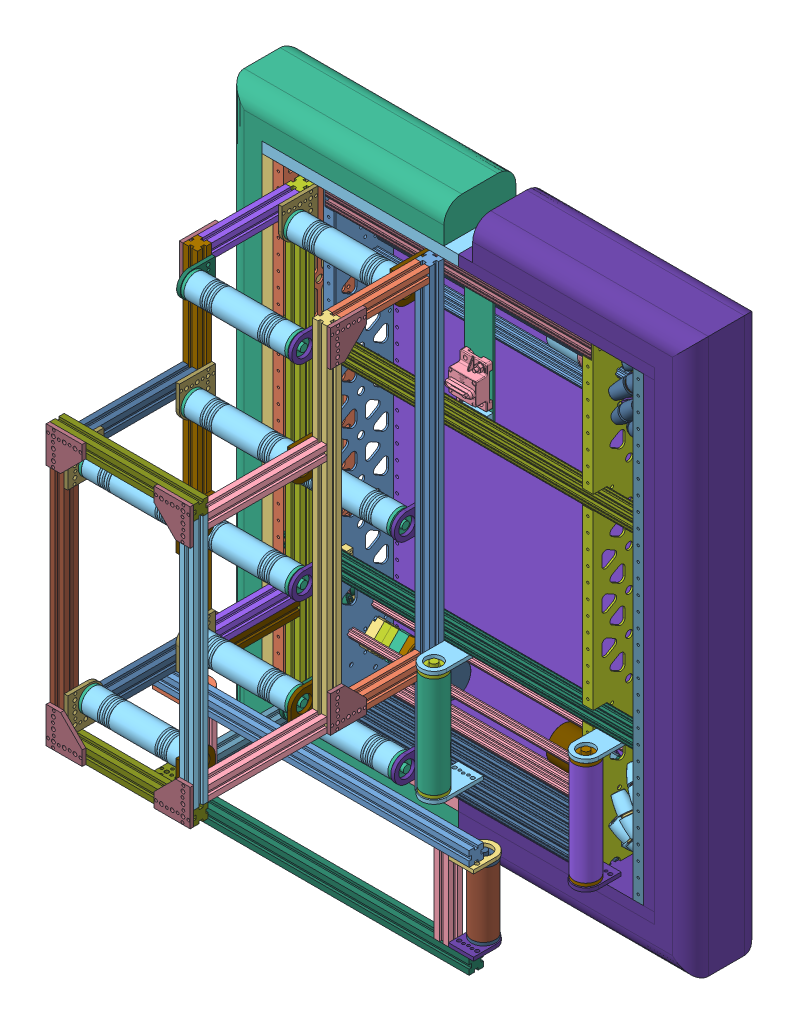
SolidWorks assembly Robot 2020, configuration Default. Lengths in mm. (continued)
Components (placement in the parent): (continued)
- Copy of Fame 2020-1: Copy of Fame 2020 [Default] at origin size (819.15 977.9 171.99) (continued)
  - NEO Gearbox 2-stage Custom v5(Mirror)^Copy of Fame 2020-1: NEO Gearbox 2-stage Custom v5(Mirror)^Copy of Fame 2020 [Default] at (0 0 425) x (-1 0 0) z (0 0 -1) size (164.9 90.53 90.53) (virtual) (continued)
    - VersaPlanetary_4_1_Gear_Kit_217-2818 v1(Mirror)^NEO Gearbox 2-stage Custom v5(Mirror)_Copy of Fame 2020-1: VersaPlanetary_4_1_Gear_Kit_217-2818 v1(Mirror)^NEO Gearbox 2-stage Custom v5(Mirror)_Copy of Fame 2020 [Default] at (-15.25 22.225 0) x (0 -0.707107 -0.707107) z (1 0 0) size (35.49 35.49 17.4) (virtual) (continued)
      - 217-2725-002 Rev1_24t Planet(Mirror)^VersaPlanetary_4_1_Gear_Kit_217-2818 v1(Mirror)_NEO Gearbox 2-stage Custom v5(Mirror)_Copy of Fame 2020-1: 217-2725-002 Rev1_24t Planet(Mirror)^VersaPlanetary_4_1_Gear_Kit_217-2818 v1(Mirror)_NEO Gearbox 2-stage Custom v5(Mirror)_Copy of Fame 2020 [Default] at (-45.2382 -525.6819 212.025) x (-0.793353 0.608761 0) z (0 0 -1) size (13.12 13.1 8) (virtual)
      - 217-2725-002 Rev1_24t Planet(Mirror)^VersaPlanetary_4_1_Gear_Kit_217-2818 v1(Mirror)_NEO Gearbox 2-stage Custom v5(Mirror)_Copy of Fame 2020-2: 217-2725-002 Rev1_24t Planet(Mirror)^VersaPlanetary_4_1_Gear_Kit_217-2818 v1(Mirror)_NEO Gearbox 2-stage Custom v5(Mirror)_Copy of Fame 2020 [Default] at (-28.1418 -525.6819 212.025) x (-0.608761 -0.793353 0) z (0 0 -1) size (13.12 13.1 8) (virtual)
      - 217-2725-002 Rev1_24t Planet(Mirror)^VersaPlanetary_4_1_Gear_Kit_217-2818 v1(Mirror)_NEO Gearbox 2-stage Custom v5(Mirror)_Copy of Fame 2020-3: 217-2725-002 Rev1_24t Planet(Mirror)^VersaPlanetary_4_1_Gear_Kit_217-2818 v1(Mirror)_NEO Gearbox 2-stage Custom v5(Mirror)_Copy of Fame 2020 [Default] at (-28.1418 -508.5855 212.025) x (0.793353 -0.608761 0) z (0 0 -1) size (13.12 13.1 8) (virtual)
      - 217-2725-002 Rev1_24t Planet(Mirror)^VersaPlanetary_4_1_Gear_Kit_217-2818 v1(Mirror)_NEO Gearbox 2-stage Custom v5(Mirror)_Copy of Fame 2020-4: 217-2725-002 Rev1_24t Planet(Mirror)^VersaPlanetary_4_1_Gear_Kit_217-2818 v1(Mirror)_NEO Gearbox 2-stage Custom v5(Mirror)_Copy of Fame 2020 [Default] at (-45.2382 -508.5855 212.025) x (0.608761 0.793353 0) z (0 0 -1) size (13.12 13.1 8) (virtual)
      - 217-2724-002 Rev1(Mirror)^VersaPlanetary_4_1_Gear_Kit_217-2818 v1(Mirror)_NEO Gearbox 2-stage Custom v5(Mirror)_Copy of Fame 2020-1: 217-2724-002 Rev1(Mirror)^VersaPlanetary_4_1_Gear_Kit_217-2818 v1(Mirror)_NEO Gearbox 2-stage Custom v5(Mirror)_Copy of Fame 2020 [Default] at (-36.69 -517.1337 218.375) x (1 0 0) z (0 0 -1) size (34.7 34.7 4.7) (virtual)
      - 217-2625-010 Rev1(Mirror)^VersaPlanetary_4_1_Gear_Kit_217-2818 v1(Mirror)_NEO Gearbox 2-stage Custom v5(Mirror)_Copy of Fame 2020-1: 217-2625-010 Rev1(Mirror)^VersaPlanetary_4_1_Gear_Kit_217-2818 v1(Mirror)_NEO Gearbox 2-stage Custom v5(Mirror)_Copy of Fame 2020 [Default] at (-45.2382 -525.6819 214.725) x (0.854322 0.519745 0) z (0 0 1) size (4 4 12) (virtual)
      - 217-2625-010 Rev1(Mirror)^VersaPlanetary_4_1_Gear_Kit_217-2818 v1(Mirror)_NEO Gearbox 2-stage Custom v5(Mirror)_Copy of Fame 2020-2: 217-2625-010 Rev1(Mirror)^VersaPlanetary_4_1_Gear_Kit_217-2818 v1(Mirror)_NEO Gearbox 2-stage Custom v5(Mirror)_Copy of Fame 2020 [Default] at (-28.1418 -525.6819 214.725) x (-0.519745 0.854322 0) z (0 0 1) size (4 4 12) (virtual)
      - 217-2625-010 Rev1(Mirror)^VersaPlanetary_4_1_Gear_Kit_217-2818 v1(Mirror)_NEO Gearbox 2-stage Custom v5(Mirror)_Copy of Fame 2020-3: 217-2625-010 Rev1(Mirror)^VersaPlanetary_4_1_Gear_Kit_217-2818 v1(Mirror)_NEO Gearbox 2-stage Custom v5(Mirror)_Copy of Fame 2020 [Default] at (-28.1418 -508.5855 214.725) x (-0.854322 -0.519745 0) z (0 0 1) size (4 4 12) (virtual)
      - 217-2625-010 Rev1(Mirror)^VersaPlanetary_4_1_Gear_Kit_217-2818 v1(Mirror)_NEO Gearbox 2-stage Custom v5(Mirror)_Copy of Fame 2020-4: 217-2625-010 Rev1(Mirror)^VersaPlanetary_4_1_Gear_Kit_217-2818 v1(Mirror)_NEO Gearbox 2-stage Custom v5(Mirror)_Copy of Fame 2020 [Default] at (-45.2382 -508.5855 214.725) x (0.519745 -0.854322 0) z (0 0 1) size (4 4 12) (virtual)
    - 217-2625-026 Rev1(Mirror)^NEO Gearbox 2-stage Custom v5(Mirror)_Copy of Fame 2020-1: 217-2625-026 Rev1(Mirror)^NEO Gearbox 2-stage Custom v5(Mirror)_Copy of Fame 2020 [Default] at (211.875 -317.5 391.6125) x (0 -0.707107 -0.707107) z (1 0 0) size (44.45 42 18.12) (virtual)
    - 217-2742-001 Rev4(Mirror)^NEO Gearbox 2-stage Custom v5(Mirror)_Copy of Fame 2020-1: 217-2742-001 Rev4(Mirror)^NEO Gearbox 2-stage Custom v5(Mirror)_Copy of Fame 2020 [Default] at (218.5752 -317.5 391.6125) x (1 0 0) z (0 -0.63857 0.769564) size (7 28 28) (virtual)
    - 217-2742-001 Rev4(Mirror)^NEO Gearbox 2-stage Custom v5(Mirror)_Copy of Fame 2020-2: 217-2742-001 Rev4(Mirror)^NEO Gearbox 2-stage Custom v5(Mirror)_Copy of Fame 2020 [Default] at (226.5752 -317.5 391.6125) x (1 0 0) z (0 -0.707107 0.707107) size (7 28 28) (virtual)
    - 217-2625-017 Rev1_9714K61(Mirror)^NEO Gearbox 2-stage Custom v5(Mirror)_Copy of Fame 2020-1: 217-2625-017 Rev1_9714K61(Mirror)^NEO Gearbox 2-stage Custom v5(Mirror)_Copy of Fame 2020 [Default] at (225.795 -317.6887 391.9075) x (0 0.983393 -0.181491) z (0 0.181491 0.983393) size (28.51 4.98 27.43) (virtual)
    - 217-2625-025 Rev1(Mirror)^NEO Gearbox 2-stage Custom v5(Mirror)_Copy of Fame 2020-1: 217-2625-025 Rev1(Mirror)^NEO Gearbox 2-stage Custom v5(Mirror)_Copy of Fame 2020 [Default] at (182.475 -317.5 391.6125) x (0 -0.707107 -0.707107) z (1 0 0) size (44.45 42 18) (virtual)
    - 217-2816-001 Rev1(Mirror)^NEO Gearbox 2-stage Custom v5(Mirror)_Copy of Fame 2020-1: 217-2816-001 Rev1(Mirror)^NEO Gearbox 2-stage Custom v5(Mirror)_Copy of Fame 2020 [Default] at (212.025 -317.5 391.6125) x (0 -0.707107 -0.707107) z (-1 0 0) size (42 42 14.5) (virtual)
    - 217-2816-001 Rev1(Mirror)^NEO Gearbox 2-stage Custom v5(Mirror)_Copy of Fame 2020-2: 217-2816-001 Rev1(Mirror)^NEO Gearbox 2-stage Custom v5(Mirror)_Copy of Fame 2020 [Default] at (199.325 -317.5 391.6125) x (0 -0.707107 -0.707107) z (-1 0 0) size (42 42 14.5) (virtual)
    - 217-4649-001 Rev1(Mirror)^NEO Gearbox 2-stage Custom v5(Mirror)_Copy of Fame 2020-1: 217-4649-001 Rev1(Mirror)^NEO Gearbox 2-stage Custom v5(Mirror)_Copy of Fame 2020 [Default] at (185.629 -317.5 391.6125) x (0 -0.707107 -0.707107) z (-1 0 0) size (18 18 13) (virtual)
    - VersaPlanetary_CIM_Adapter_217-4018 v1(Mirror)^NEO Gearbox 2-stage Custom v5(Mirror)_Copy of Fame 2020-1: VersaPlanetary_CIM_Adapter_217-4018 v1(Mirror)^NEO Gearbox 2-stage Custom v5(Mirror)_Copy of Fame 2020 [Default] at (165.15 -317.5 391.6125) x (0 -0.707107 -0.707107) z (0 -0.707107 0.707107) size (64.01 21.55 64.01) (virtual)
    - NEO Motor REV-21-1650 v2(Mirror)^NEO Gearbox 2-stage Custom v5(Mirror)_Copy of Fame 2020-1: NEO Motor REV-21-1650 v2(Mirror)^NEO Gearbox 2-stage Custom v5(Mirror)_Copy of Fame 2020 [Default] at (153.625 -317.5 391.6125) x (0 -0.707107 0.707107) z (-1 0 0) size (61.14 61.02 93.25) (virtual)
    - 3_1 Output Shaft Custom v6(Mirror)^NEO Gearbox 2-stage Custom v5(Mirror)_Copy of Fame 2020-1: 3_1 Output Shaft Custom v6(Mirror)^NEO Gearbox 2-stage Custom v5(Mirror)_Copy of Fame 2020 [Default] at (211.3752 -317.5 391.6125) x (1 0 0) z (0 -0.707107 0.707107) size (48.9 34.7 34.7) (virtual)
  - Left Wheel Assembly v4(Mirror)^Copy of Fame 2020-1: Left Wheel Assembly v4(Mirror)^Copy of Fame 2020 [Default] at (-500 0 0) x (-1 0 0) z (0 0 -1) size (65.82 166.11 165.01) (virtual)
    - 6_Mecanum_Wheel_Left_217-2799 v1(Mirror)^Left Wheel Assembly v4(Mirror)_Copy of Fame 2020-1: 6_Mecanum_Wheel_Left_217-2799 v1(Mirror)^Left Wheel Assembly v4(Mirror)_Copy of Fame 2020 [Default] x (0 0 -1) z (1 0 0) size (165.01 166.11 65.82) (virtual)
      - 217-2799-001 Rev1(Mirror)^6_Mecanum_Wheel_Left_217-2799 v1(Mirror)_Left Wheel Assembly v4(Mirror)_Copy of Fame 2020-1: 217-2799-001 Rev1(Mirror)^6_Mecanum_Wheel_Left_217-2799 v1(Mirror)_Left Wheel Assembly v4(Mirror)_Copy of Fame 2020 [Default] at (33.3875 -317.5 -234.0098) x (0.707107 0.707107 0) z (0 0 1) size (95.78 100.46 28.55) (virtual)
      - 217-2799-001 Rev1(Mirror)^6_Mecanum_Wheel_Left_217-2799 v1(Mirror)_Left Wheel Assembly v4(Mirror)_Copy of Fame 2020-2: 217-2799-001 Rev1(Mirror)^6_Mecanum_Wheel_Left_217-2799 v1(Mirror)_Left Wheel Assembly v4(Mirror)_Copy of Fame 2020 [Default] at (33.3875 -317.5 -221.3098) x (-0.987688 -0.156434 0) z (0 0 -1) size (95.78 100.46 28.55) (virtual)
      - 217-2799-002 Rev1(Mirror)^6_Mecanum_Wheel_Left_217-2799 v1(Mirror)_Left Wheel Assembly v4(Mirror)_Copy of Fame 2020-1: 217-2799-002 Rev1(Mirror)^6_Mecanum_Wheel_Left_217-2799 v1(Mirror)_Left Wheel Assembly v4(Mirror)_Copy of Fame 2020 [Default] at (4.057 -346.8305 -227.6598) x (-0.707107 0.707107 0) z (0.707107 0.707107 0) size (26.84 25.39 30.1) (virtual)
      - 217-2799-002 Rev1(Mirror)^6_Mecanum_Wheel_Left_217-2799 v1(Mirror)_Left Wheel Assembly v4(Mirror)_Copy of Fame 2020-2: 217-2799-002 Rev1(Mirror)^6_Mecanum_Wheel_Left_217-2799 v1(Mirror)_Left Wheel Assembly v4(Mirror)_Copy of Fame 2020 [Default] at (-7.5815 -323.9888 -227.6598) x (-0.156434 0.987688 0) z (0.987688 0.156434 0) size (26.84 25.39 30.1) (virtual)
      - 217-2799-002 Rev1(Mirror)^6_Mecanum_Wheel_Left_217-2799 v1(Mirror)_Left Wheel Assembly v4(Mirror)_Copy of Fame 2020-3: 217-2799-002 Rev1(Mirror)^6_Mecanum_Wheel_Left_217-2799 v1(Mirror)_Left Wheel Assembly v4(Mirror)_Copy of Fame 2020 [Default] at (-3.5711 -298.6686 -227.6598) x (0.45399 0.891007 0) z (0.891007 -0.45399 0) size (26.84 25.39 30.1) (virtual)
      - 217-2799-002 Rev1(Mirror)^6_Mecanum_Wheel_Left_217-2799 v1(Mirror)_Left Wheel Assembly v4(Mirror)_Copy of Fame 2020-4: 217-2799-002 Rev1(Mirror)^6_Mecanum_Wheel_Left_217-2799 v1(Mirror)_Left Wheel Assembly v4(Mirror)_Copy of Fame 2020 [Default] at (14.5561 -280.5414 -227.6598) x (0.891007 0.45399 0) z (0.45399 -0.891007 0) size (26.84 25.39 30.1) (virtual)
      - 217-2799-002 Rev1(Mirror)^6_Mecanum_Wheel_Left_217-2799 v1(Mirror)_Left Wheel Assembly v4(Mirror)_Copy of Fame 2020-5: 217-2799-002 Rev1(Mirror)^6_Mecanum_Wheel_Left_217-2799 v1(Mirror)_Left Wheel Assembly v4(Mirror)_Copy of Fame 2020 [Default] at (39.8763 -276.531 -227.6598) x (0.987688 -0.156434 0) z (-0.156434 -0.987688 0) size (26.84 25.39 30.1) (virtual)
      - 217-2799-002 Rev1(Mirror)^6_Mecanum_Wheel_Left_217-2799 v1(Mirror)_Left Wheel Assembly v4(Mirror)_Copy of Fame 2020-6: 217-2799-002 Rev1(Mirror)^6_Mecanum_Wheel_Left_217-2799 v1(Mirror)_Left Wheel Assembly v4(Mirror)_Copy of Fame 2020 [Default] at (62.718 -288.1695 -227.6598) x (0.707107 -0.707107 0) z (-0.707107 -0.707107 0) size (26.84 25.39 30.1) (virtual)
      - 217-2799-002 Rev1(Mirror)^6_Mecanum_Wheel_Left_217-2799 v1(Mirror)_Left Wheel Assembly v4(Mirror)_Copy of Fame 2020-7: 217-2799-002 Rev1(Mirror)^6_Mecanum_Wheel_Left_217-2799 v1(Mirror)_Left Wheel Assembly v4(Mirror)_Copy of Fame 2020 [Default] at (74.3565 -311.0112 -227.6598) x (0.156434 -0.987688 0) z (-0.987688 -0.156434 0) size (26.84 25.39 30.1) (virtual)
      - 217-2799-002 Rev1(Mirror)^6_Mecanum_Wheel_Left_217-2799 v1(Mirror)_Left Wheel Assembly v4(Mirror)_Copy of Fame 2020-8: 217-2799-002 Rev1(Mirror)^6_Mecanum_Wheel_Left_217-2799 v1(Mirror)_Left Wheel Assembly v4(Mirror)_Copy of Fame 2020 [Default] at (70.3461 -336.3314 -227.6598) x (-0.45399 -0.891007 0) z (-0.891007 0.45399 0) size (26.84 25.39 30.1) (virtual)
      - 217-2799-002 Rev1(Mirror)^6_Mecanum_Wheel_Left_217-2799 v1(Mirror)_Left Wheel Assembly v4(Mirror)_Copy of Fame 2020-9: 217-2799-002 Rev1(Mirror)^6_Mecanum_Wheel_Left_217-2799 v1(Mirror)_Left Wheel Assembly v4(Mirror)_Copy of Fame 2020 [Default] at (52.2189 -354.4586 -227.6598) x (-0.891007 -0.45399 0) z (-0.45399 0.891007 0) size (26.84 25.39 30.1) (virtual)
      - 217-2799-002 Rev1(Mirror)^6_Mecanum_Wheel_Left_217-2799 v1(Mirror)_Left Wheel Assembly v4(Mirror)_Copy of Fame 2020-10: 217-2799-002 Rev1(Mirror)^6_Mecanum_Wheel_Left_217-2799 v1(Mirror)_Left Wheel Assembly v4(Mirror)_Copy of Fame 2020 [Default] at (26.8987 -358.469 -227.6598) x (-0.987688 0.156434 0) z (0.156434 0.987688 0) size (26.84 25.39 30.1) (virtual)
      - 217-2586-003 Rev2(Mirror)^6_Mecanum_Wheel_Left_217-2799 v1(Mirror)_Left Wheel Assembly v4(Mirror)_Copy of Fame 2020-1: 217-2586-003 Rev2(Mirror)^6_Mecanum_Wheel_Left_217-2799 v1(Mirror)_Left Wheel Assembly v4(Mirror)_Copy of Fame 2020 [Default] at (-13.4676 -358.6894 -223.6536) x (0.41944 0.854155 -0.30739) z (0.757674 -0.142894 0.636798) size (19.46 28.57 19.46) (virtual)
      - 217-2586-003 Rev2(Mirror)^6_Mecanum_Wheel_Left_217-2799 v1(Mirror)_Left Wheel Assembly v4(Mirror)_Copy of Fame 2020-2: 217-2586-003 Rev2(Mirror)^6_Mecanum_Wheel_Left_217-2799 v1(Mirror)_Left Wheel Assembly v4(Mirror)_Copy of Fame 2020 [Default] at (-7.8019 -364.3551 -231.666) x (0.847342 0.451134 0.280161) z (-0.17892 0.739241 -0.649238) size (19.46 28.57 19.46) (virtual)
      - 217-2586-003 Rev2(Mirror)^6_Mecanum_Wheel_Left_217-2799 v1(Mirror)_Left Wheel Assembly v4(Mirror)_Copy of Fame 2020-3: 217-2586-003 Rev2(Mirror)^6_Mecanum_Wheel_Left_217-2799 v1(Mirror)_Left Wheel Assembly v4(Mirror)_Copy of Fame 2020 [Default] at (-27.4761 -331.196 -231.666) x (0.950684 -0.13308 0.280161) z (0.289766 0.703225 -0.649238) size (19.46 28.57 19.46) (virtual)
      - 217-2586-003 Rev2(Mirror)^6_Mecanum_Wheel_Left_217-2799 v1(Mirror)_Left Wheel Assembly v4(Mirror)_Copy of Fame 2020-4: 217-2586-003 Rev2(Mirror)^6_Mecanum_Wheel_Left_217-2799 v1(Mirror)_Left Wheel Assembly v4(Mirror)_Copy of Fame 2020 [Default] at (-23.9025 -292.8056 -231.666) x (0.690897 -0.666462 0.280161) z (0.647771 0.398601 -0.649238) size (19.46 28.57 19.46) (virtual)
      - 217-2586-003 Rev2(Mirror)^6_Mecanum_Wheel_Left_217-2799 v1(Mirror)_Left Wheel Assembly v4(Mirror)_Copy of Fame 2020-5: 217-2586-003 Rev2(Mirror)^6_Mecanum_Wheel_Left_217-2799 v1(Mirror)_Left Wheel Assembly v4(Mirror)_Copy of Fame 2020 [Default] at (1.5539 -263.8475 -231.666) x (0.167211 -0.945278 0.280161) z (0.75835 -0.058276 -0.649238) size (19.46 28.57 19.46) (virtual)
      - 217-2586-003 Rev2(Mirror)^6_Mecanum_Wheel_Left_217-2799 v1(Mirror)_Left Wheel Assembly v4(Mirror)_Copy of Fame 2020-6: 217-2586-003 Rev2(Mirror)^6_Mecanum_Wheel_Left_217-2799 v1(Mirror)_Left Wheel Assembly v4(Mirror)_Copy of Fame 2020 [Default] at (39.1697 -255.3829 -231.666) x (-0.420344 -0.86303 0.280161) z (0.579264 -0.492893 -0.649238) size (19.46 28.57 19.46) (virtual)
      - 217-2586-003 Rev2(Mirror)^6_Mecanum_Wheel_Left_217-2799 v1(Mirror)_Left Wheel Assembly v4(Mirror)_Copy of Fame 2020-7: 217-2586-003 Rev2(Mirror)^6_Mecanum_Wheel_Left_217-2799 v1(Mirror)_Left Wheel Assembly v4(Mirror)_Copy of Fame 2020 [Default] at (74.5769 -270.6449 -231.666) x (-0.847342 -0.451134 0.280161) z (0.17892 -0.739241 -0.649238) size (19.46 28.57 19.46) (virtual)
      - 217-2586-003 Rev2(Mirror)^6_Mecanum_Wheel_Left_217-2799 v1(Mirror)_Left Wheel Assembly v4(Mirror)_Copy of Fame 2020-8: 217-2586-003 Rev2(Mirror)^6_Mecanum_Wheel_Left_217-2799 v1(Mirror)_Left Wheel Assembly v4(Mirror)_Copy of Fame 2020 [Default] at (94.2511 -303.804 -231.666) x (-0.950684 0.13308 0.280161) z (-0.289766 -0.703225 -0.649238) size (19.46 28.57 19.46) (virtual)
      - 217-2586-003 Rev2(Mirror)^6_Mecanum_Wheel_Left_217-2799 v1(Mirror)_Left Wheel Assembly v4(Mirror)_Copy of Fame 2020-9: 217-2586-003 Rev2(Mirror)^6_Mecanum_Wheel_Left_217-2799 v1(Mirror)_Left Wheel Assembly v4(Mirror)_Copy of Fame 2020 [Default] at (90.6775 -342.1944 -231.666) x (-0.690897 0.666462 0.280161) z (-0.647771 -0.398601 -0.649238) size (19.46 28.57 19.46) (virtual)
      - 217-2586-003 Rev2(Mirror)^6_Mecanum_Wheel_Left_217-2799 v1(Mirror)_Left Wheel Assembly v4(Mirror)_Copy of Fame 2020-10: 217-2586-003 Rev2(Mirror)^6_Mecanum_Wheel_Left_217-2799 v1(Mirror)_Left Wheel Assembly v4(Mirror)_Copy of Fame 2020 [Default] at (65.2211 -371.1525 -231.666) x (-0.167211 0.945278 0.280161) z (-0.75835 0.058276 -0.649238) size (19.46 28.57 19.46) (virtual)
      - 217-2586-003 Rev2(Mirror)^6_Mecanum_Wheel_Left_217-2799 v1(Mirror)_Left Wheel Assembly v4(Mirror)_Copy of Fame 2020-11: 217-2586-003 Rev2(Mirror)^6_Mecanum_Wheel_Left_217-2799 v1(Mirror)_Left Wheel Assembly v4(Mirror)_Copy of Fame 2020 [Default] at (27.6053 -379.6171 -231.666) x (0.420344 0.86303 0.280161) z (-0.579264 0.492893 -0.649238) size (19.46 28.57 19.46) (virtual)
      - 217-2586-003 Rev2(Mirror)^6_Mecanum_Wheel_Left_217-2799 v1(Mirror)_Left Wheel Assembly v4(Mirror)_Copy of Fame 2020-12: 217-2586-003 Rev2(Mirror)^6_Mecanum_Wheel_Left_217-2799 v1(Mirror)_Left Wheel Assembly v4(Mirror)_Copy of Fame 2020 [Default] at (-28.7296 -323.2822 -223.6536) x (0.841394 0.444485 -0.30739) z (0.52898 -0.560953 0.636798) size (19.46 28.57 19.46) (virtual)
      - 217-2586-003 Rev2(Mirror)^6_Mecanum_Wheel_Left_217-2799 v1(Mirror)_Left Wheel Assembly v4(Mirror)_Copy of Fame 2020-13: 217-2586-003 Rev2(Mirror)^6_Mecanum_Wheel_Left_217-2799 v1(Mirror)_Left Wheel Assembly v4(Mirror)_Copy of Fame 2020 [Default] at (-20.265 -285.6664 -223.6536) x (0.941964 -0.134963 -0.30739) z (0.098234 -0.764747 0.636798) size (19.46 28.57 19.46) (virtual)
      - 217-2586-003 Rev2(Mirror)^6_Mecanum_Wheel_Left_217-2799 v1(Mirror)_Left Wheel Assembly v4(Mirror)_Copy of Fame 2020-14: 217-2586-003 Rev2(Mirror)^6_Mecanum_Wheel_Left_217-2799 v1(Mirror)_Left Wheel Assembly v4(Mirror)_Copy of Fame 2020 [Default] at (8.6931 -260.21 -223.6536) x (0.682736 -0.66286 -0.30739) z (-0.370035 -0.676434 0.636798) size (19.46 28.57 19.46) (virtual)
      - 217-2586-003 Rev2(Mirror)^6_Mecanum_Wheel_Left_217-2799 v1(Mirror)_Left Wheel Assembly v4(Mirror)_Copy of Fame 2020-15: 217-2586-003 Rev2(Mirror)^6_Mecanum_Wheel_Left_217-2799 v1(Mirror)_Left Wheel Assembly v4(Mirror)_Copy of Fame 2020 [Default] at (47.0835 -256.6364 -223.6536) x (0.162726 -0.937567 -0.30739) z (-0.696962 -0.329746 0.636798) size (19.46 28.57 19.46) (virtual)
      - 217-2586-003 Rev2(Mirror)^6_Mecanum_Wheel_Left_217-2799 v1(Mirror)_Left Wheel Assembly v4(Mirror)_Copy of Fame 2020-16: 217-2586-003 Rev2(Mirror)^6_Mecanum_Wheel_Left_217-2799 v1(Mirror)_Left Wheel Assembly v4(Mirror)_Copy of Fame 2020 [Default] at (80.2426 -276.3106 -223.6536) x (-0.41944 -0.854155 -0.30739) z (-0.757674 0.142894 0.636798) size (19.46 28.57 19.46) (virtual)
      - 217-2586-003 Rev2(Mirror)^6_Mecanum_Wheel_Left_217-2799 v1(Mirror)_Left Wheel Assembly v4(Mirror)_Copy of Fame 2020-17: 217-2586-003 Rev2(Mirror)^6_Mecanum_Wheel_Left_217-2799 v1(Mirror)_Left Wheel Assembly v4(Mirror)_Copy of Fame 2020 [Default] at (95.5046 -311.7178 -223.6536) x (-0.841394 -0.444485 -0.30739) z (-0.52898 0.560953 0.636798) size (19.46 28.57 19.46) (virtual)
      - 217-2586-003 Rev2(Mirror)^6_Mecanum_Wheel_Left_217-2799 v1(Mirror)_Left Wheel Assembly v4(Mirror)_Copy of Fame 2020-18: 217-2586-003 Rev2(Mirror)^6_Mecanum_Wheel_Left_217-2799 v1(Mirror)_Left Wheel Assembly v4(Mirror)_Copy of Fame 2020 [Default] at (87.04 -349.3336 -223.6536) x (-0.941964 0.134963 -0.30739) z (-0.098234 0.764747 0.636798) size (19.46 28.57 19.46) (virtual)
      - 217-2586-003 Rev2(Mirror)^6_Mecanum_Wheel_Left_217-2799 v1(Mirror)_Left Wheel Assembly v4(Mirror)_Copy of Fame 2020-19: 217-2586-003 Rev2(Mirror)^6_Mecanum_Wheel_Left_217-2799 v1(Mirror)_Left Wheel Assembly v4(Mirror)_Copy of Fame 2020 [Default] at (58.0819 -374.79 -223.6536) x (-0.682736 0.66286 -0.30739) z (0.370035 0.676434 0.636798) size (19.46 28.57 19.46) (virtual)
      - 217-2586-003 Rev2(Mirror)^6_Mecanum_Wheel_Left_217-2799 v1(Mirror)_Left Wheel Assembly v4(Mirror)_Copy of Fame 2020-20: 217-2586-003 Rev2(Mirror)^6_Mecanum_Wheel_Left_217-2799 v1(Mirror)_Left Wheel Assembly v4(Mirror)_Copy of Fame 2020 [Default] at (19.6915 -378.3636 -223.6536) x (-0.162726 0.937567 -0.30739) z (0.696962 0.329746 0.636798) size (19.46 28.57 19.46) (virtual)
      - 217-2586-004 Rev1(Mirror)^6_Mecanum_Wheel_Left_217-2799 v1(Mirror)_Left Wheel Assembly v4(Mirror)_Copy of Fame 2020-1: 217-2586-004 Rev1(Mirror)^6_Mecanum_Wheel_Left_217-2799 v1(Mirror)_Left Wheel Assembly v4(Mirror)_Copy of Fame 2020 [Default] at (-10.3479 -361.809 -228.0654) x (-0.690521 -0.722949 0.02293) z (-0.522667 0.476807 -0.706735) size (25.9 28.58 25.9) (virtual)
      - 217-2586-004 Rev1(Mirror)^6_Mecanum_Wheel_Left_217-2799 v1(Mirror)_Left Wheel Assembly v4(Mirror)_Copy of Fame 2020-2: 217-2586-004 Rev1(Mirror)^6_Mecanum_Wheel_Left_217-2799 v1(Mirror)_Left Wheel Assembly v4(Mirror)_Copy of Fame 2020 [Default] at (-10.9209 -361.2361 -227.2551) x (0.01458 -0.811521 0.584142) z (0.865903 0.302381 0.39847) size (25.9 28.58 25.9) (virtual)
      - 217-2586-004 Rev1(Mirror)^6_Mecanum_Wheel_Left_217-2799 v1(Mirror)_Left Wheel Assembly v4(Mirror)_Copy of Fame 2020-3: 217-2586-004 Rev1(Mirror)^6_Mecanum_Wheel_Left_217-2799 v1(Mirror)_Left Wheel Assembly v4(Mirror)_Copy of Fame 2020 [Default] at (-28.1662 -326.8394 -227.2551) x (-0.465204 -0.665104 0.584142) z (0.878265 -0.264334 0.39847) size (25.9 28.58 25.9) (virtual)
      - 217-2586-004 Rev1(Mirror)^6_Mecanum_Wheel_Left_217-2799 v1(Mirror)_Left Wheel Assembly v4(Mirror)_Copy of Fame 2020-4: 217-2586-004 Rev1(Mirror)^6_Mecanum_Wheel_Left_217-2799 v1(Mirror)_Left Wheel Assembly v4(Mirror)_Copy of Fame 2020 [Default] at (-21.9 -288.8754 -227.2551) x (-0.767297 -0.26464 0.584142) z (0.55516 -0.730082 0.39847) size (25.9 28.58 25.9) (virtual)
      - 217-2586-004 Rev1(Mirror)^6_Mecanum_Wheel_Left_217-2799 v1(Mirror)_Left Wheel Assembly v4(Mirror)_Copy of Fame 2020-5: 217-2586-004 Rev1(Mirror)^6_Mecanum_Wheel_Left_217-2799 v1(Mirror)_Left Wheel Assembly v4(Mirror)_Copy of Fame 2020 [Default] at (5.484 -261.845 -227.2551) x (-0.776308 0.236907 0.584142) z (0.020002 -0.916963 0.39847) size (25.9 28.58 25.9) (virtual)
      - 217-2586-004 Rev1(Mirror)^6_Mecanum_Wheel_Left_217-2799 v1(Mirror)_Left Wheel Assembly v4(Mirror)_Copy of Fame 2020-6: 217-2586-004 Rev1(Mirror)^6_Mecanum_Wheel_Left_217-2799 v1(Mirror)_Left Wheel Assembly v4(Mirror)_Copy of Fame 2020 [Default] at (43.5263 -256.0729 -227.2551) x (-0.488796 0.647964 0.584142) z (-0.522795 -0.753596 0.39847) size (25.9 28.58 25.9) (virtual)
      - 217-2586-004 Rev1(Mirror)^6_Mecanum_Wheel_Left_217-2799 v1(Mirror)_Left Wheel Assembly v4(Mirror)_Copy of Fame 2020-7: 217-2586-004 Rev1(Mirror)^6_Mecanum_Wheel_Left_217-2799 v1(Mirror)_Left Wheel Assembly v4(Mirror)_Copy of Fame 2020 [Default] at (77.6959 -273.7639 -227.2551) x (-0.01458 0.811521 0.584142) z (-0.865903 -0.302381 0.39847) size (25.9 28.58 25.9) (virtual)
      - 217-2586-004 Rev1(Mirror)^6_Mecanum_Wheel_Left_217-2799 v1(Mirror)_Left Wheel Assembly v4(Mirror)_Copy of Fame 2020-8: 217-2586-004 Rev1(Mirror)^6_Mecanum_Wheel_Left_217-2799 v1(Mirror)_Left Wheel Assembly v4(Mirror)_Copy of Fame 2020 [Default] at (94.9412 -308.1606 -227.2551) x (0.465204 0.665104 0.584142) z (-0.878265 0.264334 0.39847) size (25.9 28.58 25.9) (virtual)
      - 217-2586-004 Rev1(Mirror)^6_Mecanum_Wheel_Left_217-2799 v1(Mirror)_Left Wheel Assembly v4(Mirror)_Copy of Fame 2020-9: 217-2586-004 Rev1(Mirror)^6_Mecanum_Wheel_Left_217-2799 v1(Mirror)_Left Wheel Assembly v4(Mirror)_Copy of Fame 2020 [Default] at (88.675 -346.1246 -227.2551) x (0.767297 0.26464 0.584142) z (-0.55516 0.730082 0.39847) size (25.9 28.58 25.9) (virtual)
      - 217-2586-004 Rev1(Mirror)^6_Mecanum_Wheel_Left_217-2799 v1(Mirror)_Left Wheel Assembly v4(Mirror)_Copy of Fame 2020-10: 217-2586-004 Rev1(Mirror)^6_Mecanum_Wheel_Left_217-2799 v1(Mirror)_Left Wheel Assembly v4(Mirror)_Copy of Fame 2020 [Default] at (61.291 -373.155 -227.2551) x (0.776308 -0.236907 0.584142) z (-0.020002 0.916963 0.39847) size (25.9 28.58 25.9) (virtual)
      - 217-2586-004 Rev1(Mirror)^6_Mecanum_Wheel_Left_217-2799 v1(Mirror)_Left Wheel Assembly v4(Mirror)_Copy of Fame 2020-11: 217-2586-004 Rev1(Mirror)^6_Mecanum_Wheel_Left_217-2799 v1(Mirror)_Left Wheel Assembly v4(Mirror)_Copy of Fame 2020 [Default] at (23.2487 -378.9271 -227.2551) x (0.488796 -0.647964 0.584142) z (0.522795 0.753596 0.39847) size (25.9 28.58 25.9) (virtual)
      - 217-2586-004 Rev1(Mirror)^6_Mecanum_Wheel_Left_217-2799 v1(Mirror)_Left Wheel Assembly v4(Mirror)_Copy of Fame 2020-12: 217-2586-004 Rev1(Mirror)^6_Mecanum_Wheel_Left_217-2799 v1(Mirror)_Left Wheel Assembly v4(Mirror)_Copy of Fame 2020 [Default] at (-28.0394 -327.6397 -228.0654) x (-0.983582 -0.179 0.02293) z (-0.142587 0.692961 -0.706735) size (25.9 28.58 25.9) (virtual)
      - 217-2586-004 Rev1(Mirror)^6_Mecanum_Wheel_Left_217-2799 v1(Mirror)_Left Wheel Assembly v4(Mirror)_Copy of Fame 2020-13: 217-2586-004 Rev1(Mirror)^6_Mecanum_Wheel_Left_217-2799 v1(Mirror)_Left Wheel Assembly v4(Mirror)_Copy of Fame 2020 [Default] at (-22.2679 -289.5974 -228.0654) x (-0.900948 0.433321 0.02293) z (0.291957 0.644427 -0.706735) size (25.9 28.58 25.9) (virtual)
      - 217-2586-004 Rev1(Mirror)^6_Mecanum_Wheel_Left_217-2799 v1(Mirror)_Left Wheel Assembly v4(Mirror)_Copy of Fame 2020-14: 217-2586-004 Rev1(Mirror)^6_Mecanum_Wheel_Left_217-2799 v1(Mirror)_Left Wheel Assembly v4(Mirror)_Copy of Fame 2020 [Default] at (4.7621 -262.2129 -228.0654) x (-0.474183 0.880128 0.02293) z (0.614983 0.349745 -0.706735) size (25.9 28.58 25.9) (virtual)
      - 217-2586-004 Rev1(Mirror)^6_Mecanum_Wheel_Left_217-2799 v1(Mirror)_Left Wheel Assembly v4(Mirror)_Copy of Fame 2020-15: 217-2586-004 Rev1(Mirror)^6_Mecanum_Wheel_Left_217-2799 v1(Mirror)_Left Wheel Assembly v4(Mirror)_Copy of Fame 2020 [Default] at (42.726 -255.9462 -228.0654) x (0.133704 0.990756 0.02293) z (0.703107 -0.078529 -0.706735) size (25.9 28.58 25.9) (virtual)
      - 217-2586-004 Rev1(Mirror)^6_Mecanum_Wheel_Left_217-2799 v1(Mirror)_Left Wheel Assembly v4(Mirror)_Copy of Fame 2020-16: 217-2586-004 Rev1(Mirror)^6_Mecanum_Wheel_Left_217-2799 v1(Mirror)_Left Wheel Assembly v4(Mirror)_Copy of Fame 2020 [Default] at (77.1229 -273.191 -228.0654) x (0.690521 0.722949 0.02293) z (0.522667 -0.476807 -0.706735) size (25.9 28.58 25.9) (virtual)
      - 217-2586-004 Rev1(Mirror)^6_Mecanum_Wheel_Left_217-2799 v1(Mirror)_Left Wheel Assembly v4(Mirror)_Copy of Fame 2020-17: 217-2586-004 Rev1(Mirror)^6_Mecanum_Wheel_Left_217-2799 v1(Mirror)_Left Wheel Assembly v4(Mirror)_Copy of Fame 2020 [Default] at (94.8144 -307.3603 -228.0654) x (0.983582 0.179 0.02293) z (0.142587 -0.692961 -0.706735) size (25.9 28.58 25.9) (virtual)
      - 217-2586-004 Rev1(Mirror)^6_Mecanum_Wheel_Left_217-2799 v1(Mirror)_Left Wheel Assembly v4(Mirror)_Copy of Fame 2020-18: 217-2586-004 Rev1(Mirror)^6_Mecanum_Wheel_Left_217-2799 v1(Mirror)_Left Wheel Assembly v4(Mirror)_Copy of Fame 2020 [Default] at (89.0429 -345.4026 -228.0654) x (0.900948 -0.433321 0.02293) z (-0.291957 -0.644427 -0.706735) size (25.9 28.58 25.9) (virtual)
      - 217-2586-004 Rev1(Mirror)^6_Mecanum_Wheel_Left_217-2799 v1(Mirror)_Left Wheel Assembly v4(Mirror)_Copy of Fame 2020-19: 217-2586-004 Rev1(Mirror)^6_Mecanum_Wheel_Left_217-2799 v1(Mirror)_Left Wheel Assembly v4(Mirror)_Copy of Fame 2020 [Default] at (62.0129 -372.7871 -228.0654) x (0.474183 -0.880128 0.02293) z (-0.614983 -0.349745 -0.706735) size (25.9 28.58 25.9) (virtual)
      - 217-2586-004 Rev1(Mirror)^6_Mecanum_Wheel_Left_217-2799 v1(Mirror)_Left Wheel Assembly v4(Mirror)_Copy of Fame 2020-20: 217-2586-004 Rev1(Mirror)^6_Mecanum_Wheel_Left_217-2799 v1(Mirror)_Left Wheel Assembly v4(Mirror)_Copy of Fame 2020 [Default] at (24.049 -379.0538 -228.0654) x (-0.133704 -0.990756 0.02293) z (-0.703107 0.078529 -0.706735) size (25.9 28.58 25.9) (virtual)
      - 217-2586-007 Rev1(Mirror)^6_Mecanum_Wheel_Left_217-2799 v1(Mirror)_Left Wheel Assembly v4(Mirror)_Copy of Fame 2020-1: 217-2586-007 Rev1(Mirror)^6_Mecanum_Wheel_Left_217-2799 v1(Mirror)_Left Wheel Assembly v4(Mirror)_Copy of Fame 2020 [Default] at (-10.6347 -361.5222 -227.6598) x (0.5 -0.5 -0.707107) z (0.709055 0.705148 0.002763) size (61.72 5 5) (virtual)
      - 217-2586-007 Rev1(Mirror)^6_Mecanum_Wheel_Left_217-2799 v1(Mirror)_Left Wheel Assembly v4(Mirror)_Copy of Fame 2020-2: 217-2586-007 Rev1(Mirror)^6_Mecanum_Wheel_Left_217-2799 v1(Mirror)_Left Wheel Assembly v4(Mirror)_Copy of Fame 2020 [Default] at (-28.1029 -327.2391 -227.6598) x (0.110616 -0.698401 -0.707107) z (0.988113 0.153705 0.002763) size (61.72 5 5) (virtual)
      - 217-2586-007 Rev1(Mirror)^6_Mecanum_Wheel_Left_217-2799 v1(Mirror)_Left Wheel Assembly v4(Mirror)_Copy of Fame 2020-3: 217-2586-007 Rev1(Mirror)^6_Mecanum_Wheel_Left_217-2799 v1(Mirror)_Left Wheel Assembly v4(Mirror)_Copy of Fame 2020 [Default] at (-22.0838 -289.236 -227.6598) x (-0.32102 -0.630037 -0.707107) z (0.889746 -0.456448 0.002763) size (61.72 5 5) (virtual)
      - 217-2586-007 Rev1(Mirror)^6_Mecanum_Wheel_Left_217-2799 v1(Mirror)_Left Wheel Assembly v4(Mirror)_Copy of Fame 2020-4: 217-2586-007 Rev1(Mirror)^6_Mecanum_Wheel_Left_217-2799 v1(Mirror)_Left Wheel Assembly v4(Mirror)_Copy of Fame 2020 [Default] at (5.1235 -262.0287 -227.6598) x (-0.630037 -0.32102 -0.707107) z (0.451526 -0.892254 0.002763) size (61.72 5 5) (virtual)
      - 217-2586-007 Rev1(Mirror)^6_Mecanum_Wheel_Left_217-2799 v1(Mirror)_Left Wheel Assembly v4(Mirror)_Copy of Fame 2020-5: 217-2586-007 Rev1(Mirror)^6_Mecanum_Wheel_Left_217-2799 v1(Mirror)_Left Wheel Assembly v4(Mirror)_Copy of Fame 2020 [Default] at (43.1266 -256.0096 -227.6598) x (-0.698401 0.110616 -0.707107) z (-0.159162 -0.987249 0.002763) size (61.72 5 5) (virtual)
      - 217-2586-007 Rev1(Mirror)^6_Mecanum_Wheel_Left_217-2799 v1(Mirror)_Left Wheel Assembly v4(Mirror)_Copy of Fame 2020-6: 217-2586-007 Rev1(Mirror)^6_Mecanum_Wheel_Left_217-2799 v1(Mirror)_Left Wheel Assembly v4(Mirror)_Copy of Fame 2020 [Default] at (77.4097 -273.4778 -227.6598) x (-0.5 0.5 -0.707107) z (-0.709055 -0.705148 0.002763) size (61.72 5 5) (virtual)
      - 217-2586-007 Rev1(Mirror)^6_Mecanum_Wheel_Left_217-2799 v1(Mirror)_Left Wheel Assembly v4(Mirror)_Copy of Fame 2020-7: 217-2586-007 Rev1(Mirror)^6_Mecanum_Wheel_Left_217-2799 v1(Mirror)_Left Wheel Assembly v4(Mirror)_Copy of Fame 2020 [Default] at (94.8779 -307.7609 -227.6598) x (-0.110616 0.698401 -0.707107) z (-0.988113 -0.153705 0.002763) size (61.72 5 5) (virtual)
      - 217-2586-007 Rev1(Mirror)^6_Mecanum_Wheel_Left_217-2799 v1(Mirror)_Left Wheel Assembly v4(Mirror)_Copy of Fame 2020-8: 217-2586-007 Rev1(Mirror)^6_Mecanum_Wheel_Left_217-2799 v1(Mirror)_Left Wheel Assembly v4(Mirror)_Copy of Fame 2020 [Default] at (88.8588 -345.764 -227.6598) x (0.32102 0.630037 -0.707107) z (-0.889746 0.456448 0.002763) size (61.72 5 5) (virtual)
      - 217-2586-007 Rev1(Mirror)^6_Mecanum_Wheel_Left_217-2799 v1(Mirror)_Left Wheel Assembly v4(Mirror)_Copy of Fame 2020-9: 217-2586-007 Rev1(Mirror)^6_Mecanum_Wheel_Left_217-2799 v1(Mirror)_Left Wheel Assembly v4(Mirror)_Copy of Fame 2020 [Default] at (61.6515 -372.9713 -227.6598) x (0.630037 0.32102 -0.707107) z (-0.451526 0.892254 0.002763) size (61.72 5 5) (virtual)
      - 217-2586-007 Rev1(Mirror)^6_Mecanum_Wheel_Left_217-2799 v1(Mirror)_Left Wheel Assembly v4(Mirror)_Copy of Fame 2020-10: 217-2586-007 Rev1(Mirror)^6_Mecanum_Wheel_Left_217-2799 v1(Mirror)_Left Wheel Assembly v4(Mirror)_Copy of Fame 2020 [Default] at (23.6484 -378.9904 -227.6598) x (0.698401 -0.110616 -0.707107) z (0.159162 0.987249 0.002763) size (61.72 5 5) (virtual)
      - 217-2586-008 Rev1(Mirror)^6_Mecanum_Wheel_Left_217-2799 v1(Mirror)_Left Wheel Assembly v4(Mirror)_Copy of Fame 2020-1: 217-2586-008 Rev1(Mirror)^6_Mecanum_Wheel_Left_217-2799 v1(Mirror)_Left Wheel Assembly v4(Mirror)_Copy of Fame 2020 [Default] at (53.3583 -330.4692 -227.5328) x (0.544639 0.838671 0) z (0 0 -1) size (7.33 6.35 31.75) (virtual)
      - 217-2586-008 Rev1(Mirror)^6_Mecanum_Wheel_Left_217-2799 v1(Mirror)_Left Wheel Assembly v4(Mirror)_Copy of Fame 2020-2: 217-2586-008 Rev1(Mirror)^6_Mecanum_Wheel_Left_217-2799 v1(Mirror)_Left Wheel Assembly v4(Mirror)_Copy of Fame 2020 [Default] at (32.1413 -341.2799 -227.5328) x (0.99863 -0.052336 0) z (0 0 -1) size (7.33 6.35 31.75) (virtual)
      - 217-2586-008 Rev1(Mirror)^6_Mecanum_Wheel_Left_217-2799 v1(Mirror)_Left Wheel Assembly v4(Mirror)_Copy of Fame 2020-3: 217-2586-008 Rev1(Mirror)^6_Mecanum_Wheel_Left_217-2799 v1(Mirror)_Left Wheel Assembly v4(Mirror)_Copy of Fame 2020 [Default] at (12.1704 -328.3106 -227.5328) x (0.45399 -0.891007 0) z (0 0 -1) size (7.33 6.35 31.75) (virtual)
      - 217-2586-008 Rev1(Mirror)^6_Mecanum_Wheel_Left_217-2799 v1(Mirror)_Left Wheel Assembly v4(Mirror)_Copy of Fame 2020-4: 217-2586-008 Rev1(Mirror)^6_Mecanum_Wheel_Left_217-2799 v1(Mirror)_Left Wheel Assembly v4(Mirror)_Copy of Fame 2020 [Default] at (13.4167 -304.5308 -227.5328) x (-0.544639 -0.838671 0) z (0 0 -1) size (7.33 6.35 31.75) (virtual)
      - 217-2586-008 Rev1(Mirror)^6_Mecanum_Wheel_Left_217-2799 v1(Mirror)_Left Wheel Assembly v4(Mirror)_Copy of Fame 2020-5: 217-2586-008 Rev1(Mirror)^6_Mecanum_Wheel_Left_217-2799 v1(Mirror)_Left Wheel Assembly v4(Mirror)_Copy of Fame 2020 [Default] at (34.6337 -293.7201 -227.5328) x (-0.99863 0.052336 0) z (0 0 -1) size (7.33 6.35 31.75) (virtual)
      - 217-2586-008 Rev1(Mirror)^6_Mecanum_Wheel_Left_217-2799 v1(Mirror)_Left Wheel Assembly v4(Mirror)_Copy of Fame 2020-6: 217-2586-008 Rev1(Mirror)^6_Mecanum_Wheel_Left_217-2799 v1(Mirror)_Left Wheel Assembly v4(Mirror)_Copy of Fame 2020 [Default] at (54.6046 -306.6894 -227.5328) x (-0.45399 0.891007 0) z (0 0 -1) size (7.33 6.35 31.75) (virtual)
      - NUT-832-NYLOCK(Mirror)^6_Mecanum_Wheel_Left_217-2799 v1(Mirror)_Left Wheel Assembly v4(Mirror)_Copy of Fame 2020-1: NUT-832-NYLOCK(Mirror)^6_Mecanum_Wheel_Left_217-2799 v1(Mirror)_Left Wheel Assembly v4(Mirror)_Copy of Fame 2020 [Default] at (6.1639 -290.2764 -241.3161) x (0.258819 -0.965926 0) z (0.965926 0.258819 0) size (9.37 5.86 8.12) (virtual)
      - NUT-832-NYLOCK(Mirror)^6_Mecanum_Wheel_Left_217-2799 v1(Mirror)_Left Wheel Assembly v4(Mirror)_Copy of Fame 2020-2: NUT-832-NYLOCK(Mirror)^6_Mecanum_Wheel_Left_217-2799 v1(Mirror)_Left Wheel Assembly v4(Mirror)_Copy of Fame 2020 [Default] at (-0.9163 -334.9786 -241.3161) x (0.99863 -0.052336 0) z (0.052336 0.99863 0) size (9.37 5.86 8.12) (virtual)
      - NUT-832-NYLOCK(Mirror)^6_Mecanum_Wheel_Left_217-2799 v1(Mirror)_Left Wheel Assembly v4(Mirror)_Copy of Fame 2020-3: NUT-832-NYLOCK(Mirror)^6_Mecanum_Wheel_Left_217-2799 v1(Mirror)_Left Wheel Assembly v4(Mirror)_Copy of Fame 2020 [Default] at (39.4102 -355.526 -241.3161) x (0.358368 0.93358 0) z (-0.93358 0.358368 0) size (9.37 5.86 8.12) (virtual)
      - NUT-832-NYLOCK(Mirror)^6_Mecanum_Wheel_Left_217-2799 v1(Mirror)_Left Wheel Assembly v4(Mirror)_Copy of Fame 2020-4: NUT-832-NYLOCK(Mirror)^6_Mecanum_Wheel_Left_217-2799 v1(Mirror)_Left Wheel Assembly v4(Mirror)_Copy of Fame 2020 [Default] at (71.4135 -323.5227 -241.3161) x (-0.777146 0.62932 0) z (-0.62932 -0.777146 0) size (9.37 5.86 8.12) (virtual)
      - NUT-832-NYLOCK(Mirror)^6_Mecanum_Wheel_Left_217-2799 v1(Mirror)_Left Wheel Assembly v4(Mirror)_Copy of Fame 2020-5: NUT-832-NYLOCK(Mirror)^6_Mecanum_Wheel_Left_217-2799 v1(Mirror)_Left Wheel Assembly v4(Mirror)_Copy of Fame 2020 [Default] at (50.8661 -283.1962 -241.3161) x (-0.838671 -0.544639 0) z (0.544639 -0.838671 0) size (9.37 5.86 8.12) (virtual)
      - SCREW-832-1250(Mirror)^6_Mecanum_Wheel_Left_217-2799 v1(Mirror)_Left Wheel Assembly v4(Mirror)_Copy of Fame 2020-1: SCREW-832-1250(Mirror)^6_Mecanum_Wheel_Left_217-2799 v1(Mirror)_Left Wheel Assembly v4(Mirror)_Copy of Fame 2020 [Default] at (6.1639 -290.2764 -212.75) x (0 0 -1) z (0.394243 -0.919006 0) size (33.96 7.92 7.92) (virtual)
      - SCREW-832-1250(Mirror)^6_Mecanum_Wheel_Left_217-2799 v1(Mirror)_Left Wheel Assembly v4(Mirror)_Copy of Fame 2020-2: SCREW-832-1250(Mirror)^6_Mecanum_Wheel_Left_217-2799 v1(Mirror)_Left Wheel Assembly v4(Mirror)_Copy of Fame 2020 [Default] at (-0.9163 -334.9786 -212.75) x (0 0 -1) z (0.995855 0.090959 0) size (33.96 7.92 7.92) (virtual)
      - SCREW-832-1250(Mirror)^6_Mecanum_Wheel_Left_217-2799 v1(Mirror)_Left Wheel Assembly v4(Mirror)_Copy of Fame 2020-3: SCREW-832-1250(Mirror)^6_Mecanum_Wheel_Left_217-2799 v1(Mirror)_Left Wheel Assembly v4(Mirror)_Copy of Fame 2020 [Default] at (39.4102 -355.526 -212.75) x (0 0 -1) z (0.221229 0.975222 0) size (33.96 7.92 7.92) (virtual)
      - SCREW-832-1250(Mirror)^6_Mecanum_Wheel_Left_217-2799 v1(Mirror)_Left Wheel Assembly v4(Mirror)_Copy of Fame 2020-4: SCREW-832-1250(Mirror)^6_Mecanum_Wheel_Left_217-2799 v1(Mirror)_Left Wheel Assembly v4(Mirror)_Copy of Fame 2020 [Default] at (71.4135 -323.5227 -212.75) x (0 0 -1) z (-0.859128 0.511761 0) size (33.96 7.92 7.92) (virtual)
      - SCREW-832-1250(Mirror)^6_Mecanum_Wheel_Left_217-2799 v1(Mirror)_Left Wheel Assembly v4(Mirror)_Copy of Fame 2020-5: SCREW-832-1250(Mirror)^6_Mecanum_Wheel_Left_217-2799 v1(Mirror)_Left Wheel Assembly v4(Mirror)_Copy of Fame 2020 [Default] at (50.8661 -283.1962 -212.75) x (0 0 -1) z (-0.752199 -0.658936 0) size (33.96 7.92 7.92) (virtual)
      - 217-2586-005 Rev2(Mirror)^6_Mecanum_Wheel_Left_217-2799 v1(Mirror)_Left Wheel Assembly v4(Mirror)_Copy of Fame 2020-1: 217-2586-005 Rev2(Mirror)^6_Mecanum_Wheel_Left_217-2799 v1(Mirror)_Left Wheel Assembly v4(Mirror)_Copy of Fame 2020 [Default] at (-6.1597 -365.9972 -233.9884) x (-0.5 0.5 0.707107) z (-0.146447 -0.853553 0.5) size (8.5 8 8) (virtual)
      - 217-2586-005 Rev2(Mirror)^6_Mecanum_Wheel_Left_217-2799 v1(Mirror)_Left Wheel Assembly v4(Mirror)_Copy of Fame 2020-2: 217-2586-005 Rev2(Mirror)^6_Mecanum_Wheel_Left_217-2799 v1(Mirror)_Left Wheel Assembly v4(Mirror)_Copy of Fame 2020 [Default] at (-15.1097 -357.0472 -221.3312) x (-0.5 0.5 0.707107) z (-0.146447 -0.853553 0.5) size (8.5 8 8) (virtual)
      - 217-2586-005 Rev2(Mirror)^6_Mecanum_Wheel_Left_217-2799 v1(Mirror)_Left Wheel Assembly v4(Mirror)_Copy of Fame 2020-3: 217-2586-005 Rev2(Mirror)^6_Mecanum_Wheel_Left_217-2799 v1(Mirror)_Left Wheel Assembly v4(Mirror)_Copy of Fame 2020 [Default] at (-29.0929 -320.9884 -221.3312) x (-0.110616 0.698401 0.707107) z (-0.620184 -0.60446 0.5) size (8.5 8 8) (virtual)
      - 217-2586-005 Rev2(Mirror)^6_Mecanum_Wheel_Left_217-2799 v1(Mirror)_Left Wheel Assembly v4(Mirror)_Copy of Fame 2020-4: 217-2586-005 Rev2(Mirror)^6_Mecanum_Wheel_Left_217-2799 v1(Mirror)_Left Wheel Assembly v4(Mirror)_Copy of Fame 2020 [Default] at (-19.2106 -283.5972 -221.3312) x (0.32102 0.630037 0.707107) z (-0.857032 -0.124484 0.5) size (8.5 8 8) (virtual)
      - 217-2586-005 Rev2(Mirror)^6_Mecanum_Wheel_Left_217-2799 v1(Mirror)_Left Wheel Assembly v4(Mirror)_Copy of Fame 2020-5: 217-2586-005 Rev2(Mirror)^6_Mecanum_Wheel_Left_217-2799 v1(Mirror)_Left Wheel Assembly v4(Mirror)_Copy of Fame 2020 [Default] at (10.7623 -259.1556 -221.3312) x (0.630037 0.32102 0.707107) z (-0.766523 0.403042 0.5) size (8.5 8 8) (virtual)
      - 217-2586-005 Rev2(Mirror)^6_Mecanum_Wheel_Left_217-2799 v1(Mirror)_Left Wheel Assembly v4(Mirror)_Copy of Fame 2020-6: 217-2586-005 Rev2(Mirror)^6_Mecanum_Wheel_Left_217-2799 v1(Mirror)_Left Wheel Assembly v4(Mirror)_Copy of Fame 2020 [Default] at (49.3773 -256.9997 -221.3312) x (0.698401 -0.110616 0.707107) z (-0.383228 0.776618 0.5) size (8.5 8 8) (virtual)
      - 217-2586-005 Rev2(Mirror)^6_Mecanum_Wheel_Left_217-2799 v1(Mirror)_Left Wheel Assembly v4(Mirror)_Copy of Fame 2020-7: 217-2586-005 Rev2(Mirror)^6_Mecanum_Wheel_Left_217-2799 v1(Mirror)_Left Wheel Assembly v4(Mirror)_Copy of Fame 2020 [Default] at (81.8847 -277.9528 -221.3312) x (0.5 -0.5 0.707107) z (0.146447 0.853553 0.5) size (8.5 8 8) (virtual)
      - 217-2586-005 Rev2(Mirror)^6_Mecanum_Wheel_Left_217-2799 v1(Mirror)_Left Wheel Assembly v4(Mirror)_Copy of Fame 2020-8: 217-2586-005 Rev2(Mirror)^6_Mecanum_Wheel_Left_217-2799 v1(Mirror)_Left Wheel Assembly v4(Mirror)_Copy of Fame 2020 [Default] at (95.8679 -314.0116 -221.3312) x (0.110616 -0.698401 0.707107) z (0.620184 0.60446 0.5) size (8.5 8 8) (virtual)
      - 217-2586-005 Rev2(Mirror)^6_Mecanum_Wheel_Left_217-2799 v1(Mirror)_Left Wheel Assembly v4(Mirror)_Copy of Fame 2020-9: 217-2586-005 Rev2(Mirror)^6_Mecanum_Wheel_Left_217-2799 v1(Mirror)_Left Wheel Assembly v4(Mirror)_Copy of Fame 2020 [Default] at (85.9856 -351.4028 -221.3312) x (-0.32102 -0.630037 0.707107) z (0.857032 0.124484 0.5) size (8.5 8 8) (virtual)
      - 217-2586-005 Rev2(Mirror)^6_Mecanum_Wheel_Left_217-2799 v1(Mirror)_Left Wheel Assembly v4(Mirror)_Copy of Fame 2020-10: 217-2586-005 Rev2(Mirror)^6_Mecanum_Wheel_Left_217-2799 v1(Mirror)_Left Wheel Assembly v4(Mirror)_Copy of Fame 2020 [Default] at (56.0127 -375.8444 -221.3312) x (-0.630037 -0.32102 0.707107) z (0.766523 -0.403042 0.5) size (8.5 8 8) (virtual)
      - 217-2586-005 Rev2(Mirror)^6_Mecanum_Wheel_Left_217-2799 v1(Mirror)_Left Wheel Assembly v4(Mirror)_Copy of Fame 2020-11: 217-2586-005 Rev2(Mirror)^6_Mecanum_Wheel_Left_217-2799 v1(Mirror)_Left Wheel Assembly v4(Mirror)_Copy of Fame 2020 [Default] at (17.3977 -378.0003 -221.3312) x (-0.698401 0.110616 0.707107) z (0.383228 -0.776618 0.5) size (8.5 8 8) (virtual)
      - 217-2586-005 Rev2(Mirror)^6_Mecanum_Wheel_Left_217-2799 v1(Mirror)_Left Wheel Assembly v4(Mirror)_Copy of Fame 2020-12: 217-2586-005 Rev2(Mirror)^6_Mecanum_Wheel_Left_217-2799 v1(Mirror)_Left Wheel Assembly v4(Mirror)_Copy of Fame 2020 [Default] at (-27.1128 -333.4898 -233.9884) x (-0.110616 0.698401 0.707107) z (-0.620184 -0.60446 0.5) size (8.5 8 8) (virtual)
      - 217-2586-005 Rev2(Mirror)^6_Mecanum_Wheel_Left_217-2799 v1(Mirror)_Left Wheel Assembly v4(Mirror)_Copy of Fame 2020-13: 217-2586-005 Rev2(Mirror)^6_Mecanum_Wheel_Left_217-2799 v1(Mirror)_Left Wheel Assembly v4(Mirror)_Copy of Fame 2020 [Default] at (-24.9569 -294.8748 -233.9884) x (0.32102 0.630037 0.707107) z (-0.857032 -0.124484 0.5) size (8.5 8 8) (virtual)
      - 217-2586-005 Rev2(Mirror)^6_Mecanum_Wheel_Left_217-2799 v1(Mirror)_Left Wheel Assembly v4(Mirror)_Copy of Fame 2020-14: 217-2586-005 Rev2(Mirror)^6_Mecanum_Wheel_Left_217-2799 v1(Mirror)_Left Wheel Assembly v4(Mirror)_Copy of Fame 2020 [Default] at (-0.5153 -264.9019 -233.9884) x (0.630037 0.32102 0.707107) z (-0.766523 0.403042 0.5) size (8.5 8 8) (virtual)
      - 217-2586-005 Rev2(Mirror)^6_Mecanum_Wheel_Left_217-2799 v1(Mirror)_Left Wheel Assembly v4(Mirror)_Copy of Fame 2020-15: 217-2586-005 Rev2(Mirror)^6_Mecanum_Wheel_Left_217-2799 v1(Mirror)_Left Wheel Assembly v4(Mirror)_Copy of Fame 2020 [Default] at (36.8759 -255.0196 -233.9884) x (0.698401 -0.110616 0.707107) z (-0.383228 0.776618 0.5) size (8.5 8 8) (virtual)
      - 217-2586-005 Rev2(Mirror)^6_Mecanum_Wheel_Left_217-2799 v1(Mirror)_Left Wheel Assembly v4(Mirror)_Copy of Fame 2020-16: 217-2586-005 Rev2(Mirror)^6_Mecanum_Wheel_Left_217-2799 v1(Mirror)_Left Wheel Assembly v4(Mirror)_Copy of Fame 2020 [Default] at (72.9347 -269.0028 -233.9884) x (0.5 -0.5 0.707107) z (0.146447 0.853553 0.5) size (8.5 8 8) (virtual)
      - 217-2586-005 Rev2(Mirror)^6_Mecanum_Wheel_Left_217-2799 v1(Mirror)_Left Wheel Assembly v4(Mirror)_Copy of Fame 2020-17: 217-2586-005 Rev2(Mirror)^6_Mecanum_Wheel_Left_217-2799 v1(Mirror)_Left Wheel Assembly v4(Mirror)_Copy of Fame 2020 [Default] at (93.8878 -301.5102 -233.9884) x (0.110616 -0.698401 0.707107) z (0.620184 0.60446 0.5) size (8.5 8 8) (virtual)
      - 217-2586-005 Rev2(Mirror)^6_Mecanum_Wheel_Left_217-2799 v1(Mirror)_Left Wheel Assembly v4(Mirror)_Copy of Fame 2020-18: 217-2586-005 Rev2(Mirror)^6_Mecanum_Wheel_Left_217-2799 v1(Mirror)_Left Wheel Assembly v4(Mirror)_Copy of Fame 2020 [Default] at (91.7319 -340.1252 -233.9884) x (-0.32102 -0.630037 0.707107) z (0.857032 0.124484 0.5) size (8.5 8 8) (virtual)
      - 217-2586-005 Rev2(Mirror)^6_Mecanum_Wheel_Left_217-2799 v1(Mirror)_Left Wheel Assembly v4(Mirror)_Copy of Fame 2020-19: 217-2586-005 Rev2(Mirror)^6_Mecanum_Wheel_Left_217-2799 v1(Mirror)_Left Wheel Assembly v4(Mirror)_Copy of Fame 2020 [Default] at (67.2903 -370.0981 -233.9884) x (-0.630037 -0.32102 0.707107) z (0.766523 -0.403042 0.5) size (8.5 8 8) (virtual)
      - 217-2586-005 Rev2(Mirror)^6_Mecanum_Wheel_Left_217-2799 v1(Mirror)_Left Wheel Assembly v4(Mirror)_Copy of Fame 2020-20: 217-2586-005 Rev2(Mirror)^6_Mecanum_Wheel_Left_217-2799 v1(Mirror)_Left Wheel Assembly v4(Mirror)_Copy of Fame 2020 [Default] at (29.8991 -379.9804 -233.9884) x (-0.698401 0.110616 0.707107) z (0.383228 -0.776618 0.5) size (8.5 8 8) (virtual)
    - 1_2_Hex_Bore_Aluminum_VersaHub_217-2592 v1(Mirror)^Left Wheel Assembly v4(Mirror)_Copy of Fame 2020-1: 1_2_Hex_Bore_Aluminum_VersaHub_217-2592 v1(Mirror)^Left Wheel Assembly v4(Mirror)_Copy of Fame 2020 [Default] at (-239.7248 -317.5 -33.3875) x (-1 0 0) z (0 -0.707107 0.707107) size (12.7 55.88 55.88) (virtual)
  - Back Electronics Strap^Copy of Fame 2020-1: Back Electronics Strap^Copy of Fame 2020 [Default] at (0.05 266.7 84.65) x (0 1 0) z (0 0 1) size (228.6 81.6 66.64) (virtual)
